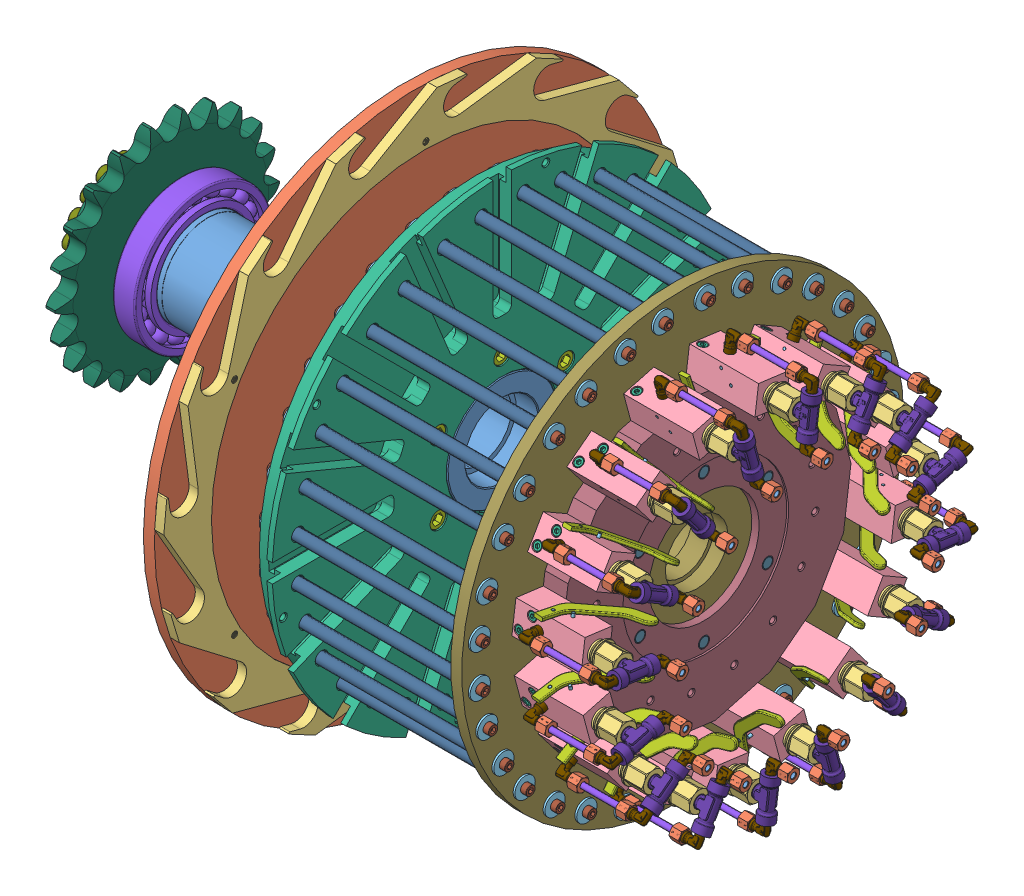
SolidWorks assembly assieme parte rotante, configuration Default. Lengths in mm. (continued)
Components (placement in the parent): (continued)
- AssiemeValvola-6: AssiemeValvola [Default] at (431.5008 -119.6927 549.8701) x (0 0.608761 -0.793353) z (0 -0.793353 -0.608761) size (90.26 138.63 38)
  - RaccordoT-1: RaccordoT [Default] at origin size (43 29.75 16.5)
  - Raccordo a L-1: Raccordo a L [Default] at (-30 0 0) x (0 -1 0) z (0 0 -1) size (28.34 25.51 14.01)
    - 1809_06_10_01-1: 1809_06_10_01 [Default] at origin size (22.49 23 10)
    - 1809_06_10_02-1: 1809_06_10_02 [Default] at origin size (6.5 8.5 8.5)
    - 1809_06_10_03-1: 1809_06_10_03 [Default] at origin size (11.02 15.01 14.01)
  - Raccordo a L-2: Raccordo a L [Default] at (30 0 0) x (0 1 0) z (0 0 -1) size (28.34 25.51 14.01)
    - 1809_06_10_01-1: 1809_06_10_01 [Default] at origin size (22.49 23 10)
    - 1809_06_10_02-1: 1809_06_10_02 [Default] at origin size (6.5 8.5 8.5)
    - 1809_06_10_03-1: 1809_06_10_03 [Default] at origin size (11.02 15.01 14.01)
  - TappoChiusura-1: TappoChiusura [Default] at (0 -32 0) x (0 -1 0) z (0 0 1) size (38.28 26.74 26.74)
  - CorpoValvola-1: CorpoValvola [Default] at (-15 -115.2824 0) size (30 75 34)
  - Raccordo a L-3: Raccordo a L [Default] at (-30 -88.2824 0) x (0 1 0) z (0 0 1) size (28.34 25.51 14.01)
    - 1809_06_10_01-1: 1809_06_10_01 [Default] at origin size (22.49 23 10)
    - 1809_06_10_02-1: 1809_06_10_02 [Default] at origin size (6.5 8.5 8.5)
    - 1809_06_10_03-1: 1809_06_10_03 [Default] at origin size (11.02 15.01 14.01)
  - Spina_3x38-1: Spina_3x38 [Default] at (0 -68.2824 -21) x (-1 0 0) z (0 0 1) size (3 3 38)
  - Spina_3x38-2: Spina_3x38 [Default] at (-10 -80.2824 -21) x (0.996193 0.087174 0) z (0 0 1) size (3 3 38)
  - M5 40mm-3: M5 40mm [ISO 4762 M5 x 40 - 40N] at (-14.6 -108.7824 9) size (45 8.5 8.5)
  - M5 40mm-2: M5 40mm [ISO 4762 M5 x 40 - 40N] at (-14.6 -96.7824 -9) size (45 8.5 8.5)
  - LevaValvola-1: LevaValvola [Default] at (-24.507 -86.571 -17) x (0.996193 0.087174 0) z (0 0 1) size (77.55 60.2 4)
  - Tubo-1: Tubo [Default] at (-30 -15.9665 0) x (1 0 0) z (0 -1 0) size (6 6 56.4)
- AssiemeValvola-7: AssiemeValvola [Default] at (431.5008 -60.2025 579.2074) x (0 0.258819 -0.965926) z (0 -0.965926 -0.258819) size (90.26 138.63 38)
  - RaccordoT-1: RaccordoT [Default] at origin size (43 29.75 16.5)
  - Raccordo a L-1: Raccordo a L [Default] at (-30 0 0) x (0 -1 0) z (0 0 -1) size (28.34 25.51 14.01)
    - 1809_06_10_01-1: 1809_06_10_01 [Default] at origin size (22.49 23 10)
    - 1809_06_10_02-1: 1809_06_10_02 [Default] at origin size (6.5 8.5 8.5)
    - 1809_06_10_03-1: 1809_06_10_03 [Default] at origin size (11.02 15.01 14.01)
  - Raccordo a L-2: Raccordo a L [Default] at (30 0 0) x (0 1 0) z (0 0 -1) size (28.34 25.51 14.01)
    - 1809_06_10_01-1: 1809_06_10_01 [Default] at origin size (22.49 23 10)
    - 1809_06_10_02-1: 1809_06_10_02 [Default] at origin size (6.5 8.5 8.5)
    - 1809_06_10_03-1: 1809_06_10_03 [Default] at origin size (11.02 15.01 14.01)
  - TappoChiusura-1: TappoChiusura [Default] at (0 -32 0) x (0 -1 0) z (0 0 1) size (38.28 26.74 26.74)
  - CorpoValvola-1: CorpoValvola [Default] at (-15 -115.2824 0) size (30 75 34)
  - Raccordo a L-3: Raccordo a L [Default] at (-30 -88.2824 0) x (0 1 0) z (0 0 1) size (28.34 25.51 14.01)
    - 1809_06_10_01-1: 1809_06_10_01 [Default] at origin size (22.49 23 10)
    - 1809_06_10_02-1: 1809_06_10_02 [Default] at origin size (6.5 8.5 8.5)
    - 1809_06_10_03-1: 1809_06_10_03 [Default] at origin size (11.02 15.01 14.01)
  - Spina_3x38-1: Spina_3x38 [Default] at (0 -68.2824 -21) x (-1 0 0) z (0 0 1) size (3 3 38)
  - Spina_3x38-2: Spina_3x38 [Default] at (-10 -80.2824 -21) x (0.996193 0.087174 0) z (0 0 1) size (3 3 38)
  - M5 40mm-3: M5 40mm [ISO 4762 M5 x 40 - 40N] at (-14.6 -108.7824 9) size (45 8.5 8.5)
  - M5 40mm-2: M5 40mm [ISO 4762 M5 x 40 - 40N] at (-14.6 -96.7824 -9) size (45 8.5 8.5)
  - LevaValvola-1: LevaValvola [Default] at (-24.507 -86.571 -17) x (0.996193 0.087174 0) z (0 0 1) size (77.55 60.2 4)
  - Tubo-1: Tubo [Default] at (-30 -15.9665 0) x (1 0 0) z (0 -1 0) size (6 6 56.4)
- AssiemeValvola-8: AssiemeValvola [Default] at (431.5008 5.9862 583.5456) x (0 -0.130526 -0.991445) z (0 -0.991445 0.130526) size (90.26 138.63 38)
  - RaccordoT-1: RaccordoT [Default] at origin size (43 29.75 16.5)
  - Raccordo a L-1: Raccordo a L [Default] at (-30 0 0) x (0 -1 0) z (0 0 -1) size (28.34 25.51 14.01)
    - 1809_06_10_01-1: 1809_06_10_01 [Default] at origin size (22.49 23 10)
    - 1809_06_10_02-1: 1809_06_10_02 [Default] at origin size (6.5 8.5 8.5)
    - 1809_06_10_03-1: 1809_06_10_03 [Default] at origin size (11.02 15.01 14.01)
  - Raccordo a L-2: Raccordo a L [Default] at (30 0 0) x (0 1 0) z (0 0 -1) size (28.34 25.51 14.01)
    - 1809_06_10_01-1: 1809_06_10_01 [Default] at origin size (22.49 23 10)
    - 1809_06_10_02-1: 1809_06_10_02 [Default] at origin size (6.5 8.5 8.5)
    - 1809_06_10_03-1: 1809_06_10_03 [Default] at origin size (11.02 15.01 14.01)
  - TappoChiusura-1: TappoChiusura [Default] at (0 -32 0) x (0 -1 0) z (0 0 1) size (38.28 26.74 26.74)
  - CorpoValvola-1: CorpoValvola [Default] at (-15 -115.2824 0) size (30 75 34)
  - Raccordo a L-3: Raccordo a L [Default] at (-30 -88.2824 0) x (0 1 0) z (0 0 1) size (28.34 25.51 14.01)
    - 1809_06_10_01-1: 1809_06_10_01 [Default] at origin size (22.49 23 10)
    - 1809_06_10_02-1: 1809_06_10_02 [Default] at origin size (6.5 8.5 8.5)
    - 1809_06_10_03-1: 1809_06_10_03 [Default] at origin size (11.02 15.01 14.01)
  - Spina_3x38-1: Spina_3x38 [Default] at (0 -68.2824 -21) x (-1 0 0) z (0 0 1) size (3 3 38)
  - Spina_3x38-2: Spina_3x38 [Default] at (-10 -80.2824 -21) x (0.996193 0.087174 0) z (0 0 1) size (3 3 38)
  - M5 40mm-3: M5 40mm [ISO 4762 M5 x 40 - 40N] at (-14.6 -108.7824 9) size (45 8.5 8.5)
  - M5 40mm-2: M5 40mm [ISO 4762 M5 x 40 - 40N] at (-14.6 -96.7824 -9) size (45 8.5 8.5)
  - LevaValvola-1: LevaValvola [Default] at (-24.507 -86.571 -17) x (0.996193 0.087174 0) z (0 0 1) size (77.55 60.2 4)
  - Tubo-1: Tubo [Default] at (-30 -15.9665 0) x (1 0 0) z (0 -1 0) size (6 6 56.4)
- AssiemeValvola-9: AssiemeValvola [Default] at (431.5008 68.7967 562.2243) x (0 -0.5 -0.866025) z (0 -0.866025 0.5) size (90.26 138.63 38)
  - RaccordoT-1: RaccordoT [Default] at origin size (43 29.75 16.5)
  - Raccordo a L-1: Raccordo a L [Default] at (-30 0 0) x (0 -1 0) z (0 0 -1) size (28.34 25.51 14.01)
    - 1809_06_10_01-1: 1809_06_10_01 [Default] at origin size (22.49 23 10)
    - 1809_06_10_02-1: 1809_06_10_02 [Default] at origin size (6.5 8.5 8.5)
    - 1809_06_10_03-1: 1809_06_10_03 [Default] at origin size (11.02 15.01 14.01)
  - Raccordo a L-2: Raccordo a L [Default] at (30 0 0) x (0 1 0) z (0 0 -1) size (28.34 25.51 14.01)
    - 1809_06_10_01-1: 1809_06_10_01 [Default] at origin size (22.49 23 10)
    - 1809_06_10_02-1: 1809_06_10_02 [Default] at origin size (6.5 8.5 8.5)
    - 1809_06_10_03-1: 1809_06_10_03 [Default] at origin size (11.02 15.01 14.01)
  - TappoChiusura-1: TappoChiusura [Default] at (0 -32 0) x (0 -1 0) z (0 0 1) size (38.28 26.74 26.74)
  - CorpoValvola-1: CorpoValvola [Default] at (-15 -115.2824 0) size (30 75 34)
  - Raccordo a L-3: Raccordo a L [Default] at (-30 -88.2824 0) x (0 1 0) z (0 0 1) size (28.34 25.51 14.01)
    - 1809_06_10_01-1: 1809_06_10_01 [Default] at origin size (22.49 23 10)
    - 1809_06_10_02-1: 1809_06_10_02 [Default] at origin size (6.5 8.5 8.5)
    - 1809_06_10_03-1: 1809_06_10_03 [Default] at origin size (11.02 15.01 14.01)
  - Spina_3x38-1: Spina_3x38 [Default] at (0 -68.2824 -21) x (-1 0 0) z (0 0 1) size (3 3 38)
  - Spina_3x38-2: Spina_3x38 [Default] at (-10 -80.2824 -21) x (0.996193 0.087174 0) z (0 0 1) size (3 3 38)
  - M5 40mm-3: M5 40mm [ISO 4762 M5 x 40 - 40N] at (-14.6 -108.7824 9) size (45 8.5 8.5)
  - M5 40mm-2: M5 40mm [ISO 4762 M5 x 40 - 40N] at (-14.6 -96.7824 -9) size (45 8.5 8.5)
  - LevaValvola-1: LevaValvola [Default] at (-24.507 -86.571 -17) x (0.996193 0.087174 0) z (0 0 1) size (77.55 60.2 4)
  - Tubo-1: Tubo [Default] at (-30 -15.9665 0) x (1 0 0) z (0 -1 0) size (6 6 56.4)
- AssiemeValvola-10: AssiemeValvola [Default] at (431.5008 118.6668 518.4894) x (0 -0.793353 -0.608761) z (0 -0.608761 0.793353) size (90.26 138.63 38)
  - RaccordoT-1: RaccordoT [Default] at origin size (43 29.75 16.5)
  - Raccordo a L-1: Raccordo a L [Default] at (-30 0 0) x (0 -1 0) z (0 0 -1) size (28.34 25.51 14.01)
    - 1809_06_10_01-1: 1809_06_10_01 [Default] at origin size (22.49 23 10)
    - 1809_06_10_02-1: 1809_06_10_02 [Default] at origin size (6.5 8.5 8.5)
    - 1809_06_10_03-1: 1809_06_10_03 [Default] at origin size (11.02 15.01 14.01)
  - Raccordo a L-2: Raccordo a L [Default] at (30 0 0) x (0 1 0) z (0 0 -1) size (28.34 25.51 14.01)
    - 1809_06_10_01-1: 1809_06_10_01 [Default] at origin size (22.49 23 10)
    - 1809_06_10_02-1: 1809_06_10_02 [Default] at origin size (6.5 8.5 8.5)
    - 1809_06_10_03-1: 1809_06_10_03 [Default] at origin size (11.02 15.01 14.01)
  - TappoChiusura-1: TappoChiusura [Default] at (0 -32 0) x (0 -1 0) z (0 0 1) size (38.28 26.74 26.74)
  - CorpoValvola-1: CorpoValvola [Default] at (-15 -115.2824 0) size (30 75 34)
  - Raccordo a L-3: Raccordo a L [Default] at (-30 -88.2824 0) x (0 1 0) z (0 0 1) size (28.34 25.51 14.01)
    - 1809_06_10_01-1: 1809_06_10_01 [Default] at origin size (22.49 23 10)
    - 1809_06_10_02-1: 1809_06_10_02 [Default] at origin size (6.5 8.5 8.5)
    - 1809_06_10_03-1: 1809_06_10_03 [Default] at origin size (11.02 15.01 14.01)
  - Spina_3x38-1: Spina_3x38 [Default] at (0 -68.2824 -21) x (-1 0 0) z (0 0 1) size (3 3 38)
  - Spina_3x38-2: Spina_3x38 [Default] at (-10 -80.2824 -21) x (0.996193 0.087174 0) z (0 0 1) size (3 3 38)
  - M5 40mm-3: M5 40mm [ISO 4762 M5 x 40 - 40N] at (-14.6 -108.7824 9) size (45 8.5 8.5)
  - M5 40mm-2: M5 40mm [ISO 4762 M5 x 40 - 40N] at (-14.6 -96.7824 -9) size (45 8.5 8.5)
  - LevaValvola-1: LevaValvola [Default] at (-24.507 -86.571 -17) x (0.996193 0.087174 0) z (0 0 1) size (77.55 60.2 4)
  - Tubo-1: Tubo [Default] at (-30 -15.9665 0) x (1 0 0) z (0 -1 0) size (6 6 56.4)
- AssiemeValvola-11: AssiemeValvola [Default] at (431.5008 148.0041 458.9992) x (0 -0.965926 -0.258819) z (0 -0.258819 0.965926) size (90.26 138.63 38)
  - RaccordoT-1: RaccordoT [Default] at origin size (43 29.75 16.5)
  - Raccordo a L-1: Raccordo a L [Default] at (-30 0 0) x (0 -1 0) z (0 0 -1) size (28.34 25.51 14.01)
    - 1809_06_10_01-1: 1809_06_10_01 [Default] at origin size (22.49 23 10)
    - 1809_06_10_02-1: 1809_06_10_02 [Default] at origin size (6.5 8.5 8.5)
    - 1809_06_10_03-1: 1809_06_10_03 [Default] at origin size (11.02 15.01 14.01)
  - Raccordo a L-2: Raccordo a L [Default] at (30 0 0) x (0 1 0) z (0 0 -1) size (28.34 25.51 14.01)
    - 1809_06_10_01-1: 1809_06_10_01 [Default] at origin size (22.49 23 10)
    - 1809_06_10_02-1: 1809_06_10_02 [Default] at origin size (6.5 8.5 8.5)
    - 1809_06_10_03-1: 1809_06_10_03 [Default] at origin size (11.02 15.01 14.01)
  - TappoChiusura-1: TappoChiusura [Default] at (0 -32 0) x (0 -1 0) z (0 0 1) size (38.28 26.74 26.74)
  - CorpoValvola-1: CorpoValvola [Default] at (-15 -115.2824 0) size (30 75 34)
  - Raccordo a L-3: Raccordo a L [Default] at (-30 -88.2824 0) x (0 1 0) z (0 0 1) size (28.34 25.51 14.01)
    - 1809_06_10_01-1: 1809_06_10_01 [Default] at origin size (22.49 23 10)
    - 1809_06_10_02-1: 1809_06_10_02 [Default] at origin size (6.5 8.5 8.5)
    - 1809_06_10_03-1: 1809_06_10_03 [Default] at origin size (11.02 15.01 14.01)
  - Spina_3x38-1: Spina_3x38 [Default] at (0 -68.2824 -21) x (-1 0 0) z (0 0 1) size (3 3 38)
  - Spina_3x38-2: Spina_3x38 [Default] at (-10 -80.2824 -21) x (0.996193 0.087174 0) z (0 0 1) size (3 3 38)
  - M5 40mm-3: M5 40mm [ISO 4762 M5 x 40 - 40N] at (-14.6 -108.7824 9) size (45 8.5 8.5)
  - M5 40mm-2: M5 40mm [ISO 4762 M5 x 40 - 40N] at (-14.6 -96.7824 -9) size (45 8.5 8.5)
  - LevaValvola-1: LevaValvola [Default] at (-24.507 -86.571 -17) x (0.996193 0.087174 0) z (0 0 1) size (77.55 60.2 4)
  - Tubo-1: Tubo [Default] at (-30 -15.9665 0) x (1 0 0) z (0 -1 0) size (6 6 56.4)
- AssiemeValvola-12: AssiemeValvola [Default] at (431.5008 152.3424 392.8105) x (0 -0.991445 0.130526) z (0 0.130526 0.991445) size (90.26 138.63 38)
  - RaccordoT-1: RaccordoT [Default] at origin size (43 29.75 16.5)
  - Raccordo a L-1: Raccordo a L [Default] at (-30 0 0) x (0 -1 0) z (0 0 -1) size (28.34 25.51 14.01)
    - 1809_06_10_01-1: 1809_06_10_01 [Default] at origin size (22.49 23 10)
    - 1809_06_10_02-1: 1809_06_10_02 [Default] at origin size (6.5 8.5 8.5)
    - 1809_06_10_03-1: 1809_06_10_03 [Default] at origin size (11.02 15.01 14.01)
  - Raccordo a L-2: Raccordo a L [Default] at (30 0 0) x (0 1 0) z (0 0 -1) size (28.34 25.51 14.01)
    - 1809_06_10_01-1: 1809_06_10_01 [Default] at origin size (22.49 23 10)
    - 1809_06_10_02-1: 1809_06_10_02 [Default] at origin size (6.5 8.5 8.5)
    - 1809_06_10_03-1: 1809_06_10_03 [Default] at origin size (11.02 15.01 14.01)
  - TappoChiusura-1: TappoChiusura [Default] at (0 -32 0) x (0 -1 0) z (0 0 1) size (38.28 26.74 26.74)
  - CorpoValvola-1: CorpoValvola [Default] at (-15 -115.2824 0) size (30 75 34)
  - Raccordo a L-3: Raccordo a L [Default] at (-30 -88.2824 0) x (0 1 0) z (0 0 1) size (28.34 25.51 14.01)
    - 1809_06_10_01-1: 1809_06_10_01 [Default] at origin size (22.49 23 10)
    - 1809_06_10_02-1: 1809_06_10_02 [Default] at origin size (6.5 8.5 8.5)
    - 1809_06_10_03-1: 1809_06_10_03 [Default] at origin size (11.02 15.01 14.01)
  - Spina_3x38-1: Spina_3x38 [Default] at (0 -68.2824 -21) x (-1 0 0) z (0 0 1) size (3 3 38)
  - Spina_3x38-2: Spina_3x38 [Default] at (-10 -80.2824 -21) x (0.996193 0.087174 0) z (0 0 1) size (3 3 38)
  - M5 40mm-3: M5 40mm [ISO 4762 M5 x 40 - 40N] at (-14.6 -108.7824 9) size (45 8.5 8.5)
  - M5 40mm-2: M5 40mm [ISO 4762 M5 x 40 - 40N] at (-14.6 -96.7824 -9) size (45 8.5 8.5)
  - LevaValvola-1: LevaValvola [Default] at (-24.507 -86.571 -17) x (0.996193 0.087174 0) z (0 0 1) size (77.55 60.2 4)
  - Tubo-1: Tubo [Default] at (-30 -15.9665 0) x (1 0 0) z (0 -1 0) size (6 6 56.4)
- AssiemeValvola-13: AssiemeValvola [Default] at (431.5008 131.0211 330) x (0 -0.866025 0.5) z (0 0.5 0.866025) size (90.26 138.63 38)
  - RaccordoT-1: RaccordoT [Default] at origin size (43 29.75 16.5)
  - Raccordo a L-1: Raccordo a L [Default] at (-30 0 0) x (0 -1 0) z (0 0 -1) size (28.34 25.51 14.01)
    - 1809_06_10_01-1: 1809_06_10_01 [Default] at origin size (22.49 23 10)
    - 1809_06_10_02-1: 1809_06_10_02 [Default] at origin size (6.5 8.5 8.5)
    - 1809_06_10_03-1: 1809_06_10_03 [Default] at origin size (11.02 15.01 14.01)
  - Raccordo a L-2: Raccordo a L [Default] at (30 0 0) x (0 1 0) z (0 0 -1) size (28.34 25.51 14.01)
    - 1809_06_10_01-1: 1809_06_10_01 [Default] at origin size (22.49 23 10)
    - 1809_06_10_02-1: 1809_06_10_02 [Default] at origin size (6.5 8.5 8.5)
    - 1809_06_10_03-1: 1809_06_10_03 [Default] at origin size (11.02 15.01 14.01)
  - TappoChiusura-1: TappoChiusura [Default] at (0 -32 0) x (0 -1 0) z (0 0 1) size (38.28 26.74 26.74)
  - CorpoValvola-1: CorpoValvola [Default] at (-15 -115.2824 0) size (30 75 34)
  - Raccordo a L-3: Raccordo a L [Default] at (-30 -88.2824 0) x (0 1 0) z (0 0 1) size (28.34 25.51 14.01)
    - 1809_06_10_01-1: 1809_06_10_01 [Default] at origin size (22.49 23 10)
    - 1809_06_10_02-1: 1809_06_10_02 [Default] at origin size (6.5 8.5 8.5)
    - 1809_06_10_03-1: 1809_06_10_03 [Default] at origin size (11.02 15.01 14.01)
  - Spina_3x38-1: Spina_3x38 [Default] at (0 -68.2824 -21) x (-1 0 0) z (0 0 1) size (3 3 38)
  - Spina_3x38-2: Spina_3x38 [Default] at (-10 -80.2824 -21) x (0.996193 0.087174 0) z (0 0 1) size (3 3 38)
  - M5 40mm-3: M5 40mm [ISO 4762 M5 x 40 - 40N] at (-14.6 -108.7824 9) size (45 8.5 8.5)
  - M5 40mm-2: M5 40mm [ISO 4762 M5 x 40 - 40N] at (-14.6 -96.7824 -9) size (45 8.5 8.5)
  - LevaValvola-1: LevaValvola [Default] at (-24.507 -86.571 -17) x (0.996193 0.087174 0) z (0 0 1) size (77.55 60.2 4)
  - Tubo-1: Tubo [Default] at (-30 -15.9665 0) x (1 0 0) z (0 -1 0) size (6 6 56.4)
- AssiemeValvola-14: AssiemeValvola [Default] at (431.5008 87.2862 280.1299) x (0 -0.608761 0.793353) z (0 0.793353 0.608761) size (90.26 138.63 38)
  - RaccordoT-1: RaccordoT [Default] at origin size (43 29.75 16.5)
  - Raccordo a L-1: Raccordo a L [Default] at (-30 0 0) x (0 -1 0) z (0 0 -1) size (28.34 25.51 14.01)
    - 1809_06_10_01-1: 1809_06_10_01 [Default] at origin size (22.49 23 10)
    - 1809_06_10_02-1: 1809_06_10_02 [Default] at origin size (6.5 8.5 8.5)
    - 1809_06_10_03-1: 1809_06_10_03 [Default] at origin size (11.02 15.01 14.01)
  - Raccordo a L-2: Raccordo a L [Default] at (30 0 0) x (0 1 0) z (0 0 -1) size (28.34 25.51 14.01)
    - 1809_06_10_01-1: 1809_06_10_01 [Default] at origin size (22.49 23 10)
    - 1809_06_10_02-1: 1809_06_10_02 [Default] at origin size (6.5 8.5 8.5)
    - 1809_06_10_03-1: 1809_06_10_03 [Default] at origin size (11.02 15.01 14.01)
  - TappoChiusura-1: TappoChiusura [Default] at (0 -32 0) x (0 -1 0) z (0 0 1) size (38.28 26.74 26.74)
  - CorpoValvola-1: CorpoValvola [Default] at (-15 -115.2824 0) size (30 75 34)
  - Raccordo a L-3: Raccordo a L [Default] at (-30 -88.2824 0) x (0 1 0) z (0 0 1) size (28.34 25.51 14.01)
    - 1809_06_10_01-1: 1809_06_10_01 [Default] at origin size (22.49 23 10)
    - 1809_06_10_02-1: 1809_06_10_02 [Default] at origin size (6.5 8.5 8.5)
    - 1809_06_10_03-1: 1809_06_10_03 [Default] at origin size (11.02 15.01 14.01)
  - Spina_3x38-1: Spina_3x38 [Default] at (0 -68.2824 -21) x (-1 0 0) z (0 0 1) size (3 3 38)
  - Spina_3x38-2: Spina_3x38 [Default] at (-10 -80.2824 -21) x (0.996193 0.087174 0) z (0 0 1) size (3 3 38)
  - M5 40mm-3: M5 40mm [ISO 4762 M5 x 40 - 40N] at (-14.6 -108.7824 9) size (45 8.5 8.5)
  - M5 40mm-2: M5 40mm [ISO 4762 M5 x 40 - 40N] at (-14.6 -96.7824 -9) size (45 8.5 8.5)
  - LevaValvola-1: LevaValvola [Default] at (-24.507 -86.571 -17) x (0.996193 0.087174 0) z (0 0 1) size (77.55 60.2 4)
  - Tubo-1: Tubo [Default] at (-30 -15.9665 0) x (1 0 0) z (0 -1 0) size (6 6 56.4)
- AssiemeValvola-15: AssiemeValvola [Default] at (431.5008 27.796 250.7926) x (0 -0.258819 0.965926) z (0 0.965926 0.258819) size (90.26 138.63 38)
  - RaccordoT-1: RaccordoT [Default] at origin size (43 29.75 16.5)
  - Raccordo a L-1: Raccordo a L [Default] at (-30 0 0) x (0 -1 0) z (0 0 -1) size (28.34 25.51 14.01)
    - 1809_06_10_01-1: 1809_06_10_01 [Default] at origin size (22.49 23 10)
    - 1809_06_10_02-1: 1809_06_10_02 [Default] at origin size (6.5 8.5 8.5)
    - 1809_06_10_03-1: 1809_06_10_03 [Default] at origin size (11.02 15.01 14.01)
  - Raccordo a L-2: Raccordo a L [Default] at (30 0 0) x (0 1 0) z (0 0 -1) size (28.34 25.51 14.01)
    - 1809_06_10_01-1: 1809_06_10_01 [Default] at origin size (22.49 23 10)
    - 1809_06_10_02-1: 1809_06_10_02 [Default] at origin size (6.5 8.5 8.5)
    - 1809_06_10_03-1: 1809_06_10_03 [Default] at origin size (11.02 15.01 14.01)
  - TappoChiusura-1: TappoChiusura [Default] at (0 -32 0) x (0 -1 0) z (0 0 1) size (38.28 26.74 26.74)
  - CorpoValvola-1: CorpoValvola [Default] at (-15 -115.2824 0) size (30 75 34)
  - Raccordo a L-3: Raccordo a L [Default] at (-30 -88.2824 0) x (0 1 0) z (0 0 1) size (28.34 25.51 14.01)
    - 1809_06_10_01-1: 1809_06_10_01 [Default] at origin size (22.49 23 10)
    - 1809_06_10_02-1: 1809_06_10_02 [Default] at origin size (6.5 8.5 8.5)
    - 1809_06_10_03-1: 1809_06_10_03 [Default] at origin size (11.02 15.01 14.01)
  - Spina_3x38-1: Spina_3x38 [Default] at (0 -68.2824 -21) x (-1 0 0) z (0 0 1) size (3 3 38)
  - Spina_3x38-2: Spina_3x38 [Default] at (-10 -80.2824 -21) x (0.996193 0.087174 0) z (0 0 1) size (3 3 38)
  - M5 40mm-3: M5 40mm [ISO 4762 M5 x 40 - 40N] at (-14.6 -108.7824 9) size (45 8.5 8.5)
  - M5 40mm-2: M5 40mm [ISO 4762 M5 x 40 - 40N] at (-14.6 -96.7824 -9) size (45 8.5 8.5)
  - LevaValvola-1: LevaValvola [Default] at (-24.507 -86.571 -17) x (0.996193 0.087174 0) z (0 0 1) size (77.55 60.2 4)
  - Tubo-1: Tubo [Default] at (-30 -15.9665 0) x (1 0 0) z (0 -1 0) size (6 6 56.4)
- AssiemeValvola-16: AssiemeValvola [Default] at (431.5008 -38.3927 246.4544) x (0 0.130526 0.991445) z (0 0.991445 -0.130526) size (90.26 138.63 38)
  - RaccordoT-1: RaccordoT [Default] at origin size (43 29.75 16.5)
  - Raccordo a L-1: Raccordo a L [Default] at (-30 0 0) x (0 -1 0) z (0 0 -1) size (28.34 25.51 14.01)
    - 1809_06_10_01-1: 1809_06_10_01 [Default] at origin size (22.49 23 10)
    - 1809_06_10_02-1: 1809_06_10_02 [Default] at origin size (6.5 8.5 8.5)
    - 1809_06_10_03-1: 1809_06_10_03 [Default] at origin size (11.02 15.01 14.01)
  - Raccordo a L-2: Raccordo a L [Default] at (30 0 0) x (0 1 0) z (0 0 -1) size (28.34 25.51 14.01)
    - 1809_06_10_01-1: 1809_06_10_01 [Default] at origin size (22.49 23 10)
    - 1809_06_10_02-1: 1809_06_10_02 [Default] at origin size (6.5 8.5 8.5)
    - 1809_06_10_03-1: 1809_06_10_03 [Default] at origin size (11.02 15.01 14.01)
  - TappoChiusura-1: TappoChiusura [Default] at (0 -32 0) x (0 -1 0) z (0 0 1) size (38.28 26.74 26.74)
  - CorpoValvola-1: CorpoValvola [Default] at (-15 -115.2824 0) size (30 75 34)
  - Raccordo a L-3: Raccordo a L [Default] at (-30 -88.2824 0) x (0 1 0) z (0 0 1) size (28.34 25.51 14.01)
    - 1809_06_10_01-1: 1809_06_10_01 [Default] at origin size (22.49 23 10)
    - 1809_06_10_02-1: 1809_06_10_02 [Default] at origin size (6.5 8.5 8.5)
    - 1809_06_10_03-1: 1809_06_10_03 [Default] at origin size (11.02 15.01 14.01)
  - Spina_3x38-1: Spina_3x38 [Default] at (0 -68.2824 -21) x (-1 0 0) z (0 0 1) size (3 3 38)
  - Spina_3x38-2: Spina_3x38 [Default] at (-10 -80.2824 -21) x (0.996193 0.087174 0) z (0 0 1) size (3 3 38)
  - M5 40mm-3: M5 40mm [ISO 4762 M5 x 40 - 40N] at (-14.6 -108.7824 9) size (45 8.5 8.5)
  - M5 40mm-2: M5 40mm [ISO 4762 M5 x 40 - 40N] at (-14.6 -96.7824 -9) size (45 8.5 8.5)
  - LevaValvola-1: LevaValvola [Default] at (-24.507 -86.571 -17) x (0.996193 0.087174 0) z (0 0 1) size (77.55 60.2 4)
  - Tubo-1: Tubo [Default] at (-30 -15.9665 0) x (1 0 0) z (0 -1 0) size (6 6 56.4)
Mates (geometry in assembly coordinates):
- Concentrico1: concentric anti-aligned: cylinder of albero rotazione piatti-1 through (-23.4119 -16.2033 415) axis (1 0 0) radius 60; cylinder of piatto rotante porta tappi-1 through (27.2184 -16.2033 415) axis (-1 0 0) radius 60
- Concentrico2: concentric aligned: circle of albero rotazione piatti-1; circle of piatto rotante porta tappi-1
- Coincidente2: coincident anti-aligned: plane of albero rotazione piatti-1 through (35.2184 -16.2033 415) normal (-1 0 0); plane of piatto rotante porta tappi-1 through (35.2184 -16.2033 415) normal (1 0 0)
- Concentrico3: concentric aligned: cylinder of piatto rotante porta tappi-1 through (35.2184 -16.2033 415) axis (-1 0 0) radius 233; cylinder of disco trasportatore tappi 31-1 through (37.2184 -16.2033 415) axis (-1 0 0) radius 233
- Coincidente4: coincident anti-aligned: plane of piatto rotante porta tappi-1 through (27.2184 -16.2033 415) normal (1 0 0); plane of disco trasportatore tappi 31-1 through (27.2184 -16.2033 415) normal (-1 0 0)
- Concentrico8: concentric aligned: cylinder of piatto rotante porta tappi-1 through (14.6994 -136.2033 622.8461) axis (1 0 0) radius 3.25; circle of disco trasportatore tappi 31-1
- Coincidente11: coincident anti-aligned: plane of albero rotazione piatti-1 through (91.2184 -16.2033 415) normal (1 0 0); plane of Disco supporto montaggio e Colonne-1 through (91.2184 -16.2033 415) normal (-1 0 0)
- Concentrico11: concentric aligned: cylinder of albero rotazione piatti-1 through (-23.4119 -16.2033 415) axis (1 0 0) radius 60; cylinder of Disco supporto montaggio e Colonne-1 through (-78.4872 -16.2033 415) axis (1 0 0) radius 60
- Concentrico12: concentric aligned: cylinder of albero rotazione piatti-1 through (17.5408 -96.2033 415) axis (1 0 0) radius 6.25; cylinder of Disco supporto montaggio e Colonne-1 through (120.2184 -96.2033 415) axis (1 0 0) radius 6.25
- Concentrico13: concentric aligned: cylinder of Disco supporto montaggio e Colonne-1 through (120.2184 -56.2033 345.718) axis (1 0 0) radius 9.25; cylinder of m12 90mm-1 through (150.9684 -56.2033 345.718) axis (1 0 0) radius 6
- Parallelo2: parallel anti-aligned: plane of m12 90mm-1 through (119.2184 -56.2033 345.718) normal (0 -1 0)
- Coincidente13: coincident anti-aligned: plane of Disco supporto montaggio e Colonne-1 through (107.2184 -56.2033 339.468) normal (1 0 0); plane of m12 90mm-1 through (107.2184 -56.2033 336.718) normal (-1 0 0)
- Concentrico17: concentric aligned: cylinder of albero rotazione piatti-1 through (-23.4119 -16.2033 415) axis (1 0 0) radius 49.75; cylinder of SKF - 6020 - 20,DE,NC,20_68-1 through (-42.4191 -16.2033 415) axis (1 0 0) radius 50
- Coincidente16: coincident anti-aligned: plane of albero rotazione piatti-1 through (-9.7816 -16.2033 415) normal (-1 0 0); plane of SKF - 6020 - 20,DE,NC,20_68-1 through (-9.7816 35.2967 415) normal (1 0 0)
- Concentrico18: concentric aligned: cylinder of albero rotazione piatti-1 through (-23.4119 -16.2033 415) axis (1 0 0) radius 50; cylinder of SKF - 6020 - 20,DE,NC,20_68-2 through (-236.6691 -16.2033 415) axis (1 0 0) radius 50
- Concentrico19: concentric anti-aligned: cylinder of albero rotazione piatti-1 through (-23.4119 -16.2033 415) axis (1 0 0) radius 48.25; cylinder of seger 100mm-1 through (-228.0316 -16.2033 415) axis (-1 0 0) radius 47.25
- Coincidente19: coincident anti-aligned: circle of albero rotazione piatti-1; plane of seger 100mm-1 through (-231.0316 -16.2033 415) normal (-1 0 0)
- Coincidente21: coincident anti-aligned: plane of albero rotazione piatti-1 through (-23.4119 -16.2033 415) normal (0 0 1); plane of seger 100mm-1 through (-231.0316 -16.2033 415) normal (0 0 -1)
- Concentrico21: concentric anti-aligned: cylinder of Disco supporto montaggio e Colonne-1 through (120.2184 124.511 241.7588) axis (1 0 0) radius 6; cylinder of asta scorrimento carello-1 through (316.2184 124.511 241.7588) axis (-1 0 0) radius 6
- Coincidente26: coincident aligned: plane of Disco supporto montaggio e Colonne-1 through (91.2184 -16.2033 415) normal (-1 0 0); plane of asta scorrimento carello-1 through (91.2184 124.511 241.7588) normal (-1 0 0)
- Concentrico22: concentric aligned: cylinder of asta scorrimento carello-1 through (91.2184 124.511 241.7588) axis (-1 0 0) radius 3.2; cylinder of M6 16mm-7 through (51.4684 124.511 241.7588) axis (-1 0 0) radius 3
- Concentrico251: concentric aligned: cylinder of asta scorrimento carello-1 through (91.2184 124.511 241.7588) axis (-1 0 0) radius 3.2; cylinder of rondella m6 22mm-1 through (56.2934 124.511 241.7588) axis (-1 0 0) radius 3.3
- Coincidente291: coincident anti-aligned: plane of asta scorrimento carello-1 through (91.2184 124.511 241.7588) normal (-1 0 0); plane of rondella m6 22mm-1 through (91.2184 121.211 241.7588) normal (1 0 0)
- Coincidente30: coincident anti-aligned: plane of M6 16mm-7 through (89.2184 119.511 241.7588) normal (1 0 0); plane of rondella m6 22mm-1 through (89.2184 113.511 241.7588) normal (-1 0 0)
- Coincidente31: coincident aligned: plane of M6 16mm-7 through (83.2184 124.511 241.7588) normal (0 -1 0); plane of rondella m6 22mm-1 through (91.2184 124.511 241.7588) normal (0 -1 0)
- Coincidente32: coincident anti-aligned: plane of asta scorrimento carello-1 through (203.7184 124.511 241.7588) normal (0 1 0); plane of M6 16mm-7 through (83.2184 124.511 241.7588) normal (0 -1 0)
- Parallelo3: parallel aligned: plane of asta scorrimento carello-1 through (203.7184 124.511 241.7588) normal (0 1 0)
- Concentrico31: concentric anti-aligned: cylinder of albero rotazione piatti-1 through (-23.4119 -16.2033 415) axis (1 0 0) radius 40; cylinder of disco trascinato porta distributore vuoto-2 through (316.2184 -16.2033 415) axis (-1 0 0) radius 30
- Coincidente37: coincident aligned: cylinder of asta scorrimento carello-23 through (91.2184 -238.2033 392) axis (1 0 0) radius 6; circle of disco trascinato porta distributore vuoto-2
- Concentrico32: concentric anti-aligned: cylinder of asta scorrimento carello-7 through (316.2184 -230.1062 351.2935) axis (-1 0 0) radius 6; circle of disco trascinato porta distributore vuoto-2
- Coincidente39: coincident anti-aligned: plane of rondella m6 22mm-42 through (316.2184 -189.4444 552.4142) normal (-1 0 0); plane of disco trascinato porta distributore vuoto-2 through (316.2184 -16.2033 415) normal (1 0 0)
- Coincidente40: coincident anti-aligned: plane of disco trascinato porta distributore vuoto-2 through (316.2184 -16.2033 415) normal (1 0 0); plane of Distributore Rotante-1 through (316.2184 -16.2033 415) normal (-1 0 0)
- Concentrico33: concentric anti-aligned: cylinder of disco trascinato porta distributore vuoto-2 through (331.2184 -16.2033 415) axis (-1 0 0) radius 67.5; cylinder of Distributore Rotante-1 through (146.5128 -16.2033 415) axis (1 0 0) radius 60
- Concentrico34: concentric aligned: cylinder of disco trascinato porta distributore vuoto-2 through (304.2184 -56.2033 345.718) axis (1 0 0) radius 6.25; circle of Distributore Rotante-1
- Concentrico35: concentric anti-aligned: cylinder of disco trascinato porta distributore vuoto-2 through (304.2184 -96.2033 415) axis (1 0 0) radius 6.25; cylinder of m12 35mm-97 through (260.4684 -96.2033 415) axis (-1 0 0) radius 6
- Coincidente41: coincident anti-aligned: plane of disco trascinato porta distributore vuoto-2 through (304.2184 -16.2033 415) normal (-1 0 0); plane of m12 35mm-97 through (304.2184 -87.2033 415) normal (1 0 0)
- Parallelo7: parallel aligned: plane of m12 35mm-97 through (292.2184 -96.2033 415) normal (0 1 0)
- Concentrico252: concentric anti-aligned: cylinder of albero rotazione piatti-1 through (-23.4119 -16.2033 415) axis (1 0 0) radius 47.5; cylinder of pulegia z =50-3 through (-217.7411 -16.2033 415) axis (-1 0 0) radius 47.5
- Coincidente292: coincident anti-aligned: plane of albero rotazione piatti-1 through (-239.7816 -16.2033 415) normal (-1 0 0); plane of pulegia z =50-3 through (-239.7816 -16.2033 415) normal (1 0 0)
- Parallelo8: parallel aligned: plane of pulegia z =50-3 through (-257.7416 -16.2033 415) normal (0 1 0)
- Concentrico253: concentric anti-aligned: cylinder of pulegia z =50-3 through (-254.7821 -16.2033 415) axis (-1 0 0) radius 67.5; cylinder of calettatore d95-1 through (-283.7821 -16.2033 415) axis (1 0 0) radius 47.5
- Coincidente294: coincident anti-aligned: plane of pulegia z =50-3 through (-254.7821 -16.2033 415) normal (-1 0 0); plane of calettatore d95-1 through (-254.7821 50.3467 415) normal (1 0 0)
- Parallelo9: parallel aligned: plane of calettatore d95-1 through (-268.7821 -16.2033 415) normal (0 1 0)
- Concentrico254: concentric anti-aligned: cylinder of piatto rotante porta tappi-1 through (14.6994 -136.2033 207.1539) axis (1 0 0) radius 3.25; cylinder of M6 20mm-1 through (-24.5316 -136.2033 207.1539) axis (-1 0 0) radius 3
- Coincidente295: coincident anti-aligned: plane of M6 20mm-1 through (13.2184 -136.2033 212.1539) normal (1 0 0); plane of rondella m6 22mm-97 through (13.2184 -147.2033 207.1539) normal (-1 0 0)
- Concentrico255: concentric aligned: cylinder of M6 20mm-1 through (-24.5316 -136.2033 207.1539) axis (-1 0 0) radius 3; cylinder of rondella m6 22mm-97 through (-19.7066 -136.2033 207.1539) axis (-1 0 0) radius 3.3
- Coincidente296: coincident anti-aligned: plane of piatto rotante porta tappi-1 through (15.2184 -16.2033 415) normal (-1 0 0); plane of rondella m6 22mm-97 through (15.2184 -139.5033 207.1539) normal (1 0 0)
- Coincidente297: coincident anti-aligned: plane of M6 20mm-1 through (7.2184 -136.2033 207.1539) normal (0 0 1); plane of rondella m6 22mm-97 through (15.2184 -136.2033 207.1539) normal (0 0 -1)
- Parallelo10: parallel aligned: plane of M6 20mm-1 through (7.2184 -136.2033 207.1539) normal (0 0 1)
- Parallelo11: parallel aligned: plane of SKF - 6020 - 20,DE,NC,20_68-1 through (-21.7816 -16.2033 415) normal (0 0 1)
- Coincidente300: coincident anti-aligned: plane of SKF - 6020 - 20,DE,NC,20_68-2 through (-228.0316 -16.2033 472.5) normal (-1 0 0); plane of seger 100mm-1 through (-228.0316 -16.2033 415) normal (1 0 0)
- Parallelo12: parallel aligned: plane of SKF - 6020 - 20,DE,NC,20_68-2 through (-216.0316 -16.2033 415) normal (0 0 1)
- Coincidente301: coincident anti-aligned: plane of disco trascinato porta distributore vuoto-2 through (316.2184 -16.2033 415) normal (1 0 0); plane of AssiemeValvola-1/CorpoValvola-1 through (316.2184 -93.9808 246.2853) normal (-1 0 0)
- Coincidente302: coincident anti-aligned: plane of Distributore Rotante-1 through (316.2184 -120.4041 296.1818) normal (0 -0.5 -0.866025); plane of AssiemeValvola-1/CorpoValvola-1 through (316.2184 -78.9808 272.2661) normal (0 0.5 0.866025)
- Concentrico256: concentric anti-aligned: circle of Distributore Rotante-1; cylinder of AssiemeValvola-1/CorpoValvola-1 through (328.7184 -93.7033 280.7661) axis (0 0.5 0.866025) radius 3
